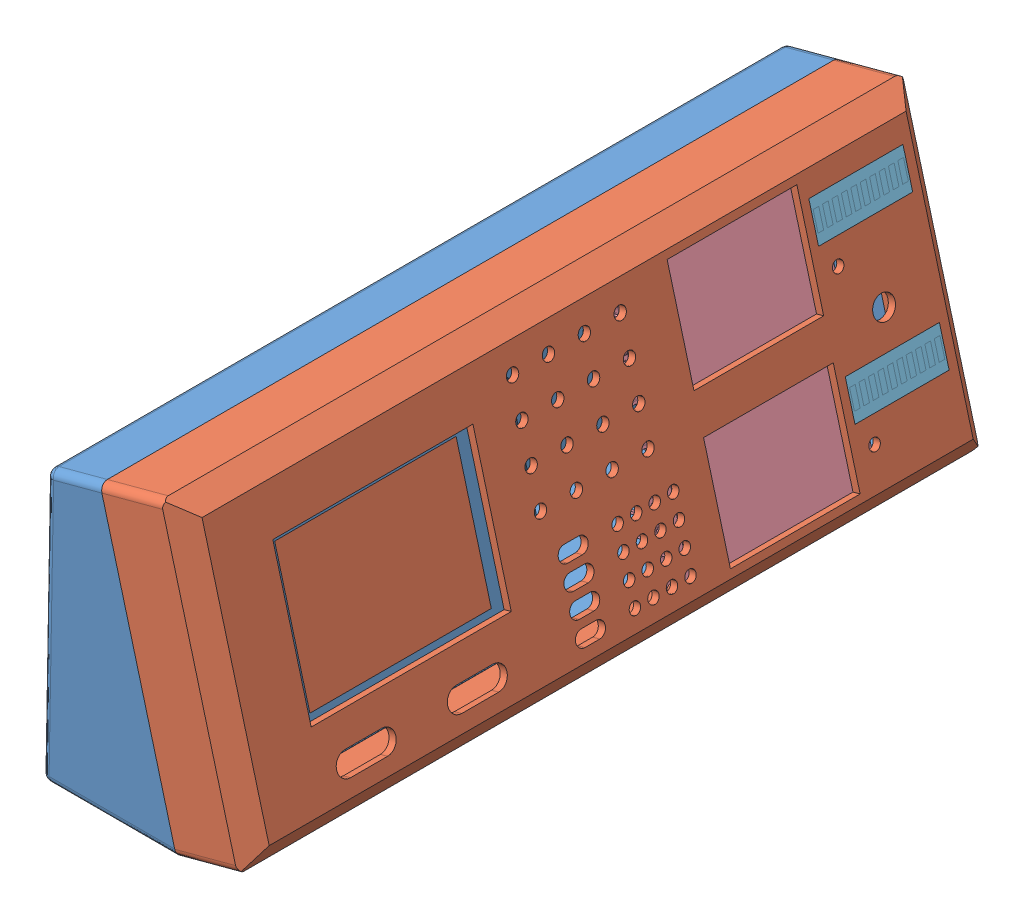
SolidWorks assembly Assem2, configuration Default. Lengths in mm.
Overall size (57.69 82.97 200).
48 component instances, 23 part files, 15 mates.
Components (placement in the parent):
- base-1: base [Default] at (69.1078 69.818 63.2839) size (36.44 77.27 200)
- front-1: front [Default] at (83.9211 91.8081 258.0277) x (0 0 -1) z (0.965926 0.258819 0) size (200 80 22)
- TFT LCD 2.4 inch ILI9341 touch-1: TFT LCD 2.4 inch ILI9341 touch [Default] at (66.1663 135.6602 172.3728) x (0 0 1) z (0.965926 0.258819 0) size (77.15 42.7 14.4)
  - TFT LCD 2.4 inch ILI9341 touch.step-1: TFT LCD 2.4 inch ILI9341 touch.step [Default] at origin size (77.15 42.7 14.4)
    - R1~R0603~R0603~HwOR.step-1: R1~R0603~R0603~HwOR.step [Default] at (51.3313 17.8702 0) x (0 -1 0) z (0 0 -1) size (1.62 0.81 0.45)
      - R0603~R0603~HwOR.step-1: R0603~R0603~HwOR.step [Default] at origin size (1.62 0.81 0.45)
    - C1~C0603~C0603_L1.6-W0.8-H0.8~HwOR.step-1: C1~C0603~C0603_L1.6-W0.8-H0.8~HwOR.step [Default] at (30.0394 8.9761 0) x (1 0 0) z (0 0 -1) size (1.6 0.8 0.8)
      - C0603~C0603_L1.6-W0.8-H0.8~HwOR.step-1: C0603~C0603_L1.6-W0.8-H0.8~HwOR.step [Default] at origin size (1.6 0.8 0.8)
    - H2~HDR-TH_4P-P2.54-V-M~HDR-TH_4P-P2.54-M-LI-1X4P~HwOR.step-1: H2~HDR-TH_4P-P2.54-V-M~HDR-TH_4P-P2.54-M-LI-1X4P~HwOR.step [Default] at (75.1801 25.1701 0) x (0 -1 0) z (0 0 -1) size (10.17 2.66 11.54)
      - HDR-TH_4P-P2.54-V-M~HDR-TH_4P-P2.54-M-LI-1X4P~HwOR.step-1: HDR-TH_4P-P2.54-V-M~HDR-TH_4P-P2.54-M-LI-1X4P~HwOR.step [Default] at origin size (10.17 2.66 11.54)
    - H3~CONN-TH_PZ254V-11-14P~CONN-TH_PZ254V-11-14P~HwOR.step-1: H3~CONN-TH_PZ254V-11-14P~CONN-TH_PZ254V-11-14P~HwOR.step [Default] at (2 4.85 0) x (0 1 0) z (0 0 -1) size (35.57 2.5 11.6)
      - CONN-TH_PZ254V-11-14P~CONN-TH_PZ254V-11-14P~HwOR.step-1: CONN-TH_PZ254V-11-14P~CONN-TH_PZ254V-11-14P~HwOR.step [Default] at origin size (35.57 2.5 11.6)
    - Q1~SOT-23-3_L2.9-W1.3-P1.90-LS2.4-BR~SOT-23-3P_L2.9-W1.3-H1.0-LS2.4-P0.95~HwOR.step-1: Q1~SOT-23-3_L2.9-W1.3-P1.90-LS2.4-BR~SOT-23-3P_L2.9-W1.3-H1.0-LS2.4-P0.95~HwOR.step [Default] at (19.5843 21.1653 0) x (-1 0 0) z (0 0 -1) size (2.5 2.89 1.06)
      - SOT-23-3_L2.9-W1.3-P1.90-LS2.4-BR~SOT-23-3P_L2.9-W1.3-H1.0-LS2.4-P0.95~HwOR.step-1: SOT-23-3_L2.9-W1.3-P1.90-LS2.4-BR~SOT-23-3P_L2.9-W1.3-H1.0-LS2.4-P0.95~HwOR.step [Default] at origin size (2.5 2.89 1.06)
    - U1~SD-CARD-SMD_SD-CARD-11P~SD-CARD-SMD_SD-CARD-11P~HwOR.step-1: U1~SD-CARD-SMD_SD-CARD-11P~SD-CARD-SMD_SD-CARD-11P~HwOR.step [Default] at (48.7311 32.7935 0) x (1 0 0) z (0 0 -1) size (27.7 17.71 3.85)
      - SD-CARD-SMD_SD-CARD-11P~SD-CARD-SMD_SD-CARD-11P~HwOR.step-1: SD-CARD-SMD_SD-CARD-11P~SD-CARD-SMD_SD-CARD-11P~HwOR.step [Default] at origin size (27.7 17.71 3.85)
    - U2~TSSOP-16_L5.0-W4.4-P0.65-LS6.4-BL~TSSOP-16_L5.0-W4.4-H1.0-LS6.4-P0.65~HwOR.step-1: U2~TSSOP-16_L5.0-W4.4-P0.65-LS6.4-BL~TSSOP-16_L5.0-W4.4-H1.0-LS6.4-P0.65~HwOR.step [Default] at (22.8993 6.6301 0) x (0 -1 0) z (0 0 -1) size (5 6.41 1.05)
      - TSSOP-16_L5.0-W4.4-P0.65-LS6.4-BL~TSSOP-16_L5.0-W4.4-H1.0-LS6.4-P0.65~HwOR.step-1: TSSOP-16_L5.0-W4.4-P0.65-LS6.4-BL~TSSOP-16_L5.0-W4.4-H1.0-LS6.4-P0.65~HwOR.step [Default] at origin size (5 6.41 1.05)
    - R1~R0603~R0603~HwOR.step-2: R1~R0603~R0603~HwOR.step [Default] at (48.6536 17.8702 0) x (0 -1 0) z (0 0 -1) size (1.62 0.81 0.45)
      - R0603~R0603~HwOR.step-1: R0603~R0603~HwOR.step [Default] at origin size (1.62 0.81 0.45)
    - R1~R0603~R0603~HwOR.step-3: R1~R0603~R0603~HwOR.step [Default] at (45.9973 17.8702 0) x (0 -1 0) z (0 0 -1) size (1.62 0.81 0.45)
      - R0603~R0603~HwOR.step-1: R0603~R0603~HwOR.step [Default] at origin size (1.62 0.81 0.45)
    - R1~R0603~R0603~HwOR.step-4: R1~R0603~R0603~HwOR.step [Default] at (16.535 21.1653 0) x (0 -1 0) z (0 0 -1) size (1.62 0.81 0.45)
      - R0603~R0603~HwOR.step-1: R0603~R0603~HwOR.step [Default] at origin size (1.62 0.81 0.45)
    - R1~R0603~R0603~HwOR.step-5: R1~R0603~R0603~HwOR.step [Default] at (16.6772 4.0801 0) x (0 -1 0) z (0 0 -1) size (1.62 0.81 0.45)
      - R0603~R0603~HwOR.step-1: R0603~R0603~HwOR.step [Default] at origin size (1.62 0.81 0.45)
    - R1~R0603~R0603~HwOR.step-6: R1~R0603~R0603~HwOR.step [Default] at (22.9395 21.1858 0) x (0 -1 0) z (0 0 -1) size (1.62 0.81 0.45)
      - R0603~R0603~HwOR.step-1: R0603~R0603~HwOR.step [Default] at origin size (1.62 0.81 0.45)
    - C1~C0603~C0603_L1.6-W0.8-H0.8~HwOR.step-2: C1~C0603~C0603_L1.6-W0.8-H0.8~HwOR.step [Default] at (22.7962 15.1258 0) x (0 -1 0) z (0 0 -1) size (1.6 0.8 0.8)
      - C0603~C0603_L1.6-W0.8-H0.8~HwOR.step-1: C0603~C0603_L1.6-W0.8-H0.8~HwOR.step [Default] at origin size (1.6 0.8 0.8)
    - Q1~SOT-23-3_L2.9-W1.3-P1.90-LS2.4-BR~SOT-23-3P_L2.9-W1.3-H1.0-LS2.4-P0.95~HwOR.step-2: Q1~SOT-23-3_L2.9-W1.3-P1.90-LS2.4-BR~SOT-23-3P_L2.9-W1.3-H1.0-LS2.4-P0.95~HwOR.step [Default] at (19.3803 15.2492 0) x (0 1 0) z (0 0 -1) size (2.5 2.89 1.06)
      - SOT-23-3_L2.9-W1.3-P1.90-LS2.4-BR~SOT-23-3P_L2.9-W1.3-H1.0-LS2.4-P0.95~HwOR.step-1: SOT-23-3_L2.9-W1.3-P1.90-LS2.4-BR~SOT-23-3P_L2.9-W1.3-H1.0-LS2.4-P0.95~HwOR.step [Default] at origin size (2.5 2.89 1.06)
    - Board~HwOR.step-1: Board~HwOR.step [Default] at origin size (77.15 42.69 1.6)
    - TopSilkscreen~HwOR.step-1: TopSilkscreen~HwOR.step [Default] at (0 0 1.6201) size (76.19 42.7 0.01)
    - BottomSilkscreen~HwOR.step-1: BottomSilkscreen~HwOR.step [Default] at (0 0 -0.02) size (75.96 41.18 0.02)
    - text.step-1: text.step [Default] at origin size (2.87 0.1 1)
    - EasyEDA PCB Model~HwOR.step-1: EasyEDA PCB Model~HwOR.step [Default] at origin size (60.51 42.69 4.2)
    - EasyEDA PCB Model~HwOR-0.step-1: EasyEDA PCB Model~HwOR-0.step [Default] at origin size (4.46 5.93 4.2)
    - EasyEDA PCB Model~HwOR-1.step-1: EasyEDA PCB Model~HwOR-1.step [Default] at origin size (4.45 0.59 4.2)
    - EasyEDA PCB Model~HwOR-2.step-1: EasyEDA PCB Model~HwOR-2.step [Default] at origin size (4.45 31.81 4.2)
    - EasyEDA PCB Model~HwOR-3.step-1: EasyEDA PCB Model~HwOR-3.step [Default] at origin size (4.45 0.62 4.2)
    - EasyEDA PCB Model~HwOR-4.step-1: EasyEDA PCB Model~HwOR-4.step [Default] at origin size (54.06 40.69 4.2)
    - EasyEDA PCB Model~HwOR-5.step-1: EasyEDA PCB Model~HwOR-5.step [Default] at origin size (48.96 36.72 4.2)
    - EasyEDA PCB Model~HwOR-6.step-1: EasyEDA PCB Model~HwOR-6.step [Default] at origin size (3.3 10.72 0.1)
- 1.8 inch TFT Display SPI-1: 1.8 inch TFT Display SPI [Default] at (64.5593 129.6805 118.615) x (0 0 1) z (0.965926 0.258819 0) size (58 34.5 12.5)
- 1.8 inch TFT Display SPI-2: 1.8 inch TFT Display SPI [Default] at (74.3944 92.9753 118.6513) x (0 0 1) z (0.965926 0.258819 0) size (58 34.5 12.5)
- LED Bar Graph Array-1: LED Bar Graph Array [Default] at (67.9417 135.6804 83.3839) x (-0.258819 0.965926 0) z (0.965926 0.258819 0) size (10.17 26.17 9.09)
- LED Bar Graph Array-2: LED Bar Graph Array [Default] at (77.7768 98.9752 83.3839) x (-0.258819 0.965926 0) z (0.965926 0.258819 0) size (10.17 26.17 9.09)
Mates (geometry in assembly coordinates):
- Coincident1: coincident anti-aligned: plane of base-1 through (48.4023 147.092 263.2839) normal (0.965926 0.258819 0); plane of front-1 through (64.6026 86.6318 258.0277) normal (-0.965926 -0.258819 0)
- Coincident2: coincident aligned: plane of base-1 through (69.1078 69.818 263.2839) normal (0 0 1); plane of front-1 through (69.1078 69.818 263.2839) normal (0 0 1)
- Coincident3: coincident aligned: plane of base-1 through (33.9134 143.2098 263.2839) normal (-0.258819 0.965926 0); plane of front-1 through (48.4023 147.092 63.2839) normal (-0.258819 0.965926 0)
- Coincident4: coincident anti-aligned: plane of front-1 through (83.9211 91.8081 258.0277) normal (-0.965926 -0.258819 0); plane of TFT LCD 2.4 inch ILI9341 touch-1/TFT LCD 2.4 inch ILI9341 touch.step-1/EasyEDA PCB Model~HwOR-5.step-1 through (77.3004 116.5169 215.8003) normal (0.965926 0.258819 0)
- Width1: width anti-aligned: plane of TFT LCD 2.4 inch ILI9341 touch-1/TFT LCD 2.4 inch ILI9341 touch.step-1/EasyEDA PCB Model~HwOR.step-1 through (78.7654 94.8222 243.177) normal (0.258819 -0.965926 0); plane of front-1 through (67.7152 136.0621 187.1166) normal (-0.258819 0.965926 0); plane of TFT LCD 2.4 inch ILI9341 touch-1/TFT LCD 2.4 inch ILI9341 touch.step-1/EasyEDA PCB Model~HwOR.step-1 through (82.4735 97.2107 242.2839) normal (-0.258819 0.965926 0); plane of front-1 through (72.1208 135.8477 242.2839) normal (0.258819 -0.965926 0)
- Coincident5: coincident anti-aligned: plane of front-1 through (83.9211 91.8081 258.0277) normal (-0.965926 -0.258819 0); plane of 1.8 inch TFT Display SPI-1 through (73.156 131.984 116.465) normal (0.965926 0.258819 0)
- Coincident6: coincident anti-aligned: plane of front-1 through (83.9211 91.8081 258.0277) normal (-0.965926 -0.258819 0); plane of 1.8 inch TFT Display SPI-2 through (82.9912 95.2788 116.5013) normal (0.965926 0.258819 0)
- Width2: width anti-aligned: plane of 1.8 inch TFT Display SPI-2 through (87.4558 78.6166 139.7013) normal (0.258819 -0.965926 0); plane of front-1 through (78.5265 111.941 139.7013) normal (-0.258819 0.965926 0); plane of 1.8 inch TFT Display SPI-2 through (86.6146 81.7558 133.2839) normal (-0.258819 0.965926 0); plane of front-1 through (79.3677 108.8018 133.2839) normal (0.258819 -0.965926 0)
- Width3: width anti-aligned: plane of 1.8 inch TFT Display SPI-1 through (77.6207 115.3218 139.665) normal (0.258819 -0.965926 0); plane of front-1 through (68.6914 148.6462 139.665) normal (-0.258819 0.965926 0); plane of 1.8 inch TFT Display SPI-1 through (76.7795 118.461 133.2839) normal (-0.258819 0.965926 0); plane of front-1 through (69.5326 145.5069 133.2839) normal (0.258819 -0.965926 0)
- Coincident8: coincident: plane of front-1 through (70.5679 141.6432 96.0839) normal (0.258819 -0.965926 0); plane of LED Bar Graph Array-1 through (72.4997 142.1609 96.0839) normal (-0.258819 0.965926 0)
- Coincident9: coincident: plane of front-1 through (80.403 104.9381 96.0839) normal (0.258819 -0.965926 0); plane of LED Bar Graph Array-2 through (82.3348 105.4557 96.0839) normal (-0.258819 0.965926 0)
- Coincident10: coincident: plane of front-1 through (83.0326 95.1243 96.0839) normal (0 0 -1); plane of LED Bar Graph Array-2 through (84.9644 95.6419 96.0839) normal (0 0 1)
- Coincident11: coincident: plane of front-1 through (73.1975 131.8294 96.0839) normal (0 0 -1); plane of LED Bar Graph Array-1 through (75.1293 132.3471 96.0839) normal (0 0 1)
- Coincident12: coincident aligned: plane of front-1 through (85.853 92.3258 258.0277) normal (0.965926 0.258819 0); plane of LED Bar Graph Array-2 through (84.9644 95.6419 70.6839) normal (0.965926 0.258819 0)
- Coincident13: coincident aligned: plane of front-1 through (85.853 92.3258 258.0277) normal (0.965926 0.258819 0); plane of LED Bar Graph Array-1 through (75.1293 132.3471 70.6839) normal (0.965926 0.258819 0)
